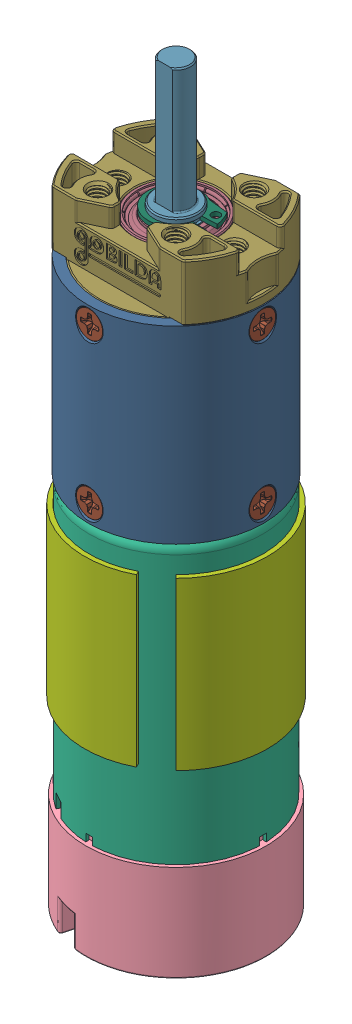
SolidWorks assembly 5202-2402-0051 moteur, configuration Défaut. Lengths in mm.
Overall size (52.36 150.75 52.36).
38 component instances, 16 part files, 0 mates.
Components (placement in the parent):
- 5202-2402-0051.step-1: 5202-2402-0051.step [Défaut] at origin size (52.36 150.75 52.36)
  - 5000-0002-0001.step-1: 5000-0002-0001.step [Défaut] at origin size (52.36 88.75 52.36)
    - 5000-0002-0001 encoder cap.step-1: 5000-0002-0001 encoder cap.step [Défaut] x (0 1 0) z (0 0 1) size (22.84 52.33 52.33)
      - JST-XH-4POS-VERT (1).step-1: JST-XH-4POS-VERT (1).step [Défaut] at (2.8 12.25 -75.95) x (1 0 0) z (0 0 -1) size (10.4 12.83 12.83)
        - Plastic (1).step-1: Plastic (1).step [Défaut] at (-6.1146 -33.6358 -52.1967) x (0 0.707107 0.707107) z (-1 0 0) size (12.4 5.75 7)
        - Pin (1).step-1: Pin (1).step [Défaut] at (-7.7146 -29.3225 -51.2067) x (0 0.707107 0.707107) z (-1 0 0) size (0.64 0.64 10)
        - Pin (1).step-2: Pin (1).step [Défaut] at (-7.7146 -34.6258 -56.51) x (0 0.707107 0.707107) z (-1 0 0) size (0.64 0.64 10)
        - Pin (1).step-3: Pin (1).step [Défaut] at (-7.7146 -32.858 -54.7423) x (0 0.707107 0.707107) z (-1 0 0) size (0.64 0.64 10)
        - Pin (1).step-4: Pin (1).step [Défaut] at (-7.7146 -31.0902 -52.9745) x (0 0.707107 0.707107) z (-1 0 0) size (0.64 0.64 10)
      - screw.step-1: screw.step [Défaut] at (-41.264 -8.1646 3.9905) x (0.882398 0 0.470504) z (0 -1 0) size (8.86 7.85 4.95)
        - 99461A915_Phillips Rounded Head Thread-Forming Screws (1).step-1: 99461A915_Phillips Rounded Head Thread-Forming Screws (1).step [Défaut] at (27.264 -14.6475 -49.347) x (-0.332697 -0.623949 0.707107) z (-0.882398 0.470504 0) size (3.5 3.5 7.4)
      - screw_1.step-1: screw_1.step [Défaut] at (-14.4172 7.3354 3.9905) x (0.882398 0 0.470504) z (0 -1 0) size (8.86 7.85 4.95)
        - 99461A915_Phillips Rounded Head Thread-Forming Screws (1).step-1: 99461A915_Phillips Rounded Head Thread-Forming Screws (1).step [Défaut] at (-10.5142 -28.4382 -25.8237) x (-0.332697 -0.623949 0.707107) z (-0.882398 0.470504 0) size (3.5 3.5 7.4)
      - endcap.step-1: endcap.step [Défaut] at (72.6354 37.1707 -11.0784) x (0 -0.707107 -0.707107) z (1 0 0) size (37 37 21.84)
      - base.step-1: base.step [Défaut] at (-55.8646 37.1707 -11.0784) x (0 -0.707107 -0.707107) z (-1 0 0) size (34.96 34.31 1)
    - 5000-0002-0001 body.step-1: 5000-0002-0001 body.step [Défaut] at (-37.1707 3.4854 -11.0784) size (35.61 61.8 35.61)
    - 5000-0002-0001 motor shield.step-1: 5000-0002-0001 motor shield.step [Défaut] at (-37.1707 54.6354 -11.0784) x (0.808104 0 -0.58904) z (0 -1 0) size (37.5 37.27 34.15)
    - 5000-0002-0001 motor shaft.step-1: 5000-0002-0001 motor shaft.step [Défaut] at (-37.1707 59.4854 -11.0784) size (3.14 12.45 3.14)
  - 5102-0024-0051.step-1: 5102-0024-0051.step [Défaut] at origin size (36 76.68 35.98)
    - 5102 Gearbox Base.step-1: 5102 Gearbox Base.step [Défaut] at (-37.1707 60.1354 -11.0784) size (31.91 5.69 31.91)
    - 5102 Gearbox Barrel (3 stage, simple)_Gear Blank.step-1: 5102 Gearbox Barrel (3 stage, simple)_Gear Blank.step [Défaut] at (-37.1707 111.8354 -11.0784) x (1 0 0) z (0 -1 0) size (35.98 35.98 38.7)
    - 5102 Gearbox Barrel Screw (M3 x 8mm length Flat Head)_92010A118.step-1: 5102 Gearbox Barrel Screw (M3 x 8mm length Flat Head)_92010A118.step [Défaut] at (-37.1707 63.6354 5.0046) x (0.002439 -0.999997 0) z (0 0 1) size (5.46 5.46 8)
    - 5102 Gearbox Face.step-1: 5102 Gearbox Face.step [Défaut] at (-37.1707 93.3354 -11.0784) size (36 17.1 31.91)
    - 5102 Gearbox Bearing.step-1: 5102 Gearbox Bearing.step [Défaut] at (-37.1707 101.4354 -11.0784) size (17 5 17)
    - 5102 Gearbox Shaft (23.5mm Length, Simple).step-1: 5102 Gearbox Shaft (23.5mm Length, Simple).step [Défaut] at (-37.1707 89.9754 -11.0784) x (0.894773 0 -0.44652) z (0.44652 0 0.894773) size (8.97 40.6 8.97)
    - 5102 Gearbox Snap Ring.step-1: 5102 Gearbox Snap Ring.step [Défaut] at (-37.1707 106.5104 -11.0784) x (0 1 0) z (0 0 1) size (0.85 13.06 10.66)
    - 5102 Gearbox Barrel Screw (M3 x 8mm length Flat Head)_92010A118.step-2: 5102 Gearbox Barrel Screw (M3 x 8mm length Flat Head)_92010A118.step [Défaut] at (-37.1707 95.3354 5.0046) x (-0.002439 -0.999997 0) z (0 0 1) size (5.46 5.46 8)
    - 5102 Gearbox Barrel Screw (M3 x 8mm length Flat Head)_92010A118.step-3: 5102 Gearbox Barrel Screw (M3 x 8mm length Flat Head)_92010A118.step [Défaut] at (-21.0877 63.6354 -11.0784) x (0 -0.999997 -0.002439) z (1 0 0) size (5.46 5.46 8)
    - 5102 Gearbox Barrel Screw (M3 x 8mm length Flat Head)_92010A118.step-4: 5102 Gearbox Barrel Screw (M3 x 8mm length Flat Head)_92010A118.step [Défaut] at (-37.1707 63.6354 -27.1614) x (-0.002439 -0.999997 0) z (0 0 -1) size (5.46 5.46 8)
    - 5102 Gearbox Barrel Screw (M3 x 8mm length Flat Head)_92010A118.step-5: 5102 Gearbox Barrel Screw (M3 x 8mm length Flat Head)_92010A118.step [Défaut] at (-53.2537 63.6354 -11.0784) x (0 -0.999997 0.002439) z (-1 0 0) size (5.46 5.46 8)
    - 5102 Gearbox Barrel Screw (M3 x 8mm length Flat Head)_92010A118.step-6: 5102 Gearbox Barrel Screw (M3 x 8mm length Flat Head)_92010A118.step [Défaut] at (-21.0877 95.3354 -11.0784) x (0 -0.999997 0.002439) z (1 0 0) size (5.46 5.46 8)
    - 5102 Gearbox Barrel Screw (M3 x 8mm length Flat Head)_92010A118.step-7: 5102 Gearbox Barrel Screw (M3 x 8mm length Flat Head)_92010A118.step [Défaut] at (-37.1707 95.3354 -27.1614) x (0.002439 -0.999997 0) z (0 0 -1) size (5.46 5.46 8)
    - 5102 Gearbox Barrel Screw (M3 x 8mm length Flat Head)_92010A118.step-8: 5102 Gearbox Barrel Screw (M3 x 8mm length Flat Head)_92010A118.step [Défaut] at (-53.2537 95.3354 -11.0784) x (0 -0.999997 -0.002439) z (-1 0 0) size (5.46 5.46 8)
    - 5102 Gearbox Bearing.step-2: 5102 Gearbox Bearing.step [Défaut] at (-37.1707 93.3354 -11.0784) size (17 5 17)
    - 5102 Gearbox Base Mounting Screw M3 x 5mm length SHCS)_91290A110.step-1: 5102 Gearbox Base Mounting Screw M3 x 5mm length SHCS)_91290A110.step [Défaut] at (-46.0096 57.2554 -2.2396) x (0.056382 0 0.998409) z (0 -1 0) size (5.5 5.5 8)
    - 5102 Gearbox Base Mounting Screw M3 x 5mm length SHCS)_91290A110.step-2: 5102 Gearbox Base Mounting Screw M3 x 5mm length SHCS)_91290A110.step [Défaut] at (-28.3319 57.2554 -2.2396) x (0.998409 0 -0.056382) z (0 -1 0) size (5.5 5.5 8)
    - 5102 Gearbox Base Mounting Screw M3 x 5mm length SHCS)_91290A110.step-3: 5102 Gearbox Base Mounting Screw M3 x 5mm length SHCS)_91290A110.step [Défaut] at (-28.3319 57.2554 -19.9173) x (-0.056382 0 -0.998409) z (0 -1 0) size (5.5 5.5 8)
    - 5102 Gearbox Base Mounting Screw M3 x 5mm length SHCS)_91290A110.step-4: 5102 Gearbox Base Mounting Screw M3 x 5mm length SHCS)_91290A110.step [Défaut] at (-46.0096 57.2554 -19.9173) x (-0.998409 0 0.056382) z (0 -1 0) size (5.5 5.5 8)
